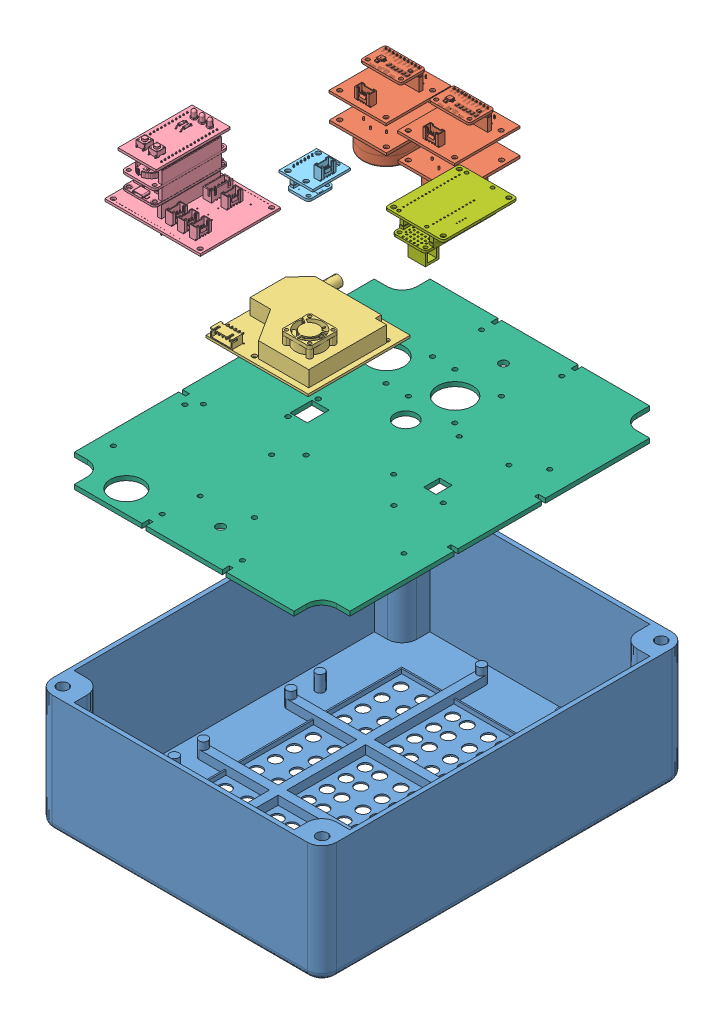
SolidWorks assembly box sizing diagram, configuration Default. Lengths in mm.
Overall size (195 398.67 250).
8 component instances, 7 part files, 15 mates.
Components (placement in the parent):
- 230x150x85 box-1: 230x150x85 box [Default] at (85.5807 -118.13 179.4613) size (195 84 250)
- gas-3: gas [Default] at (190.8291 335.5901 145.5155) x (1 0 0) z (0 0 -1) size (39.2 50.23 44.9)
- gas-4: gas [Default] at (143.7664 335.8786 145.4693) x (1 0 0) z (0 0 -1) size (39.2 50.23 44.9)
- dust sENSOR-1: dust sENSOR [Default] at (136.3641 176.0538 346.3342) x (1 0 0) z (0 1 0) size (70 72.51 20.87)
- main pcb sensors-1: main pcb sensors [Default] at (33.2021 236.8331 265.9989) x (0 0 -1) z (0 1 0) size (55.17 65.72 49.14)
- TEMPERATURE-1: TEMPERATURE [Default] at (71.1713 327.832 207.4158) x (0 0 -1) z (-1 0 0) size (25.77 23.35 23.17)
- Base plate-1: Base plate [Default] at (12.078 88.545 202.3984) size (189 3 244)
- Protomic-1: Protomic [Default] at (131.6692 265.0405 124.2988) x (0 0 -1) z (0 -1 0) size (53.4 40.03 27.15)
Mates (geometry in assembly coordinates):
- Concentric1: concentric aligned: circle of Base plate-1; circle of 230x150x85 box-1
- Concentric2: concentric anti-aligned: circle of gas-4; circle of Base plate-1
- Concentric7: concentric anti-aligned: circle of gas-3; circle of Base plate-1
- Parallel3: parallel aligned: plane of gas-3 through (68.9645 231.88 93.6112) normal (0 0 -1); plane of Base plate-1 through (12.078 91.545 57.4613) normal (0 0 -1)
- Parallel4: parallel aligned: plane of gas-4 through (21.9018 232.1685 93.565) normal (0 0 -1); plane of Base plate-1 through (12.078 91.545 57.4613) normal (0 0 -1)
- Coincident8: coincident anti-aligned: line of Base plate-1 through (146.2637 91.545 185.9556) axis (0 -1 0); line of Protomic-1 through (146.2637 248.747 185.9556) axis (0 1 0)
- Parallel5: parallel aligned: plane of Base plate-1 through (12.078 91.545 57.4613) normal (0 0 -1); plane of Protomic-1 through (129.7407 237.811 138.2455) normal (0 0 -1)
- Concentric8: concentric: circle of TEMPERATURE-1; circle of Base plate-1
- Parallel6: parallel aligned: plane of TEMPERATURE-1 through (39.8029 237.5487 190.5632) normal (-1 0 0); plane of Base plate-1 through (-8.9193 91.545 202.3984) normal (-1 0 0)
- Coincident13: coincident aligned: line of main pcb sensors-1 through (2.3239 238.4031 216.1935) axis (0 -1 0); line of Base plate-1 through (2.3239 91.545 216.1935) axis (0 -1 0)
- Parallel7: parallel aligned: plane of main pcb sensors-1 through (6.4981 242.5531 235.4689) normal (-1 0 0); plane of Base plate-1 through (-8.9193 91.545 202.3984) normal (-1 0 0)
- Concentric9: concentric aligned: circle of dust sENSOR-1; cylinder of Base plate-1 through (91.7709 91.545 259.4077) axis (0 -1 0) radius 1.6
- Parallel8: parallel aligned: plane of dust sENSOR-1 through (132.7709 187.4908 263.6077) normal (0 0 1); plane of Base plate-1 through (12.078 91.545 301.4613) normal (0 0 1)
- Parallel9: parallel aligned: line of 230x150x85 box-1 through (10.0807 -38.13 301.4613) axis (1 0 0); line of Base plate-1 through (10.2307 91.545 301.4613) axis (1 0 0)
- Parallel10: parallel aligned: line of 230x150x85 box-1 through (183.0807 -38.13 294.4613) axis (0 0 -1); line of Base plate-1 through (180.0807 91.545 282.3113) axis (0 0 -1)
